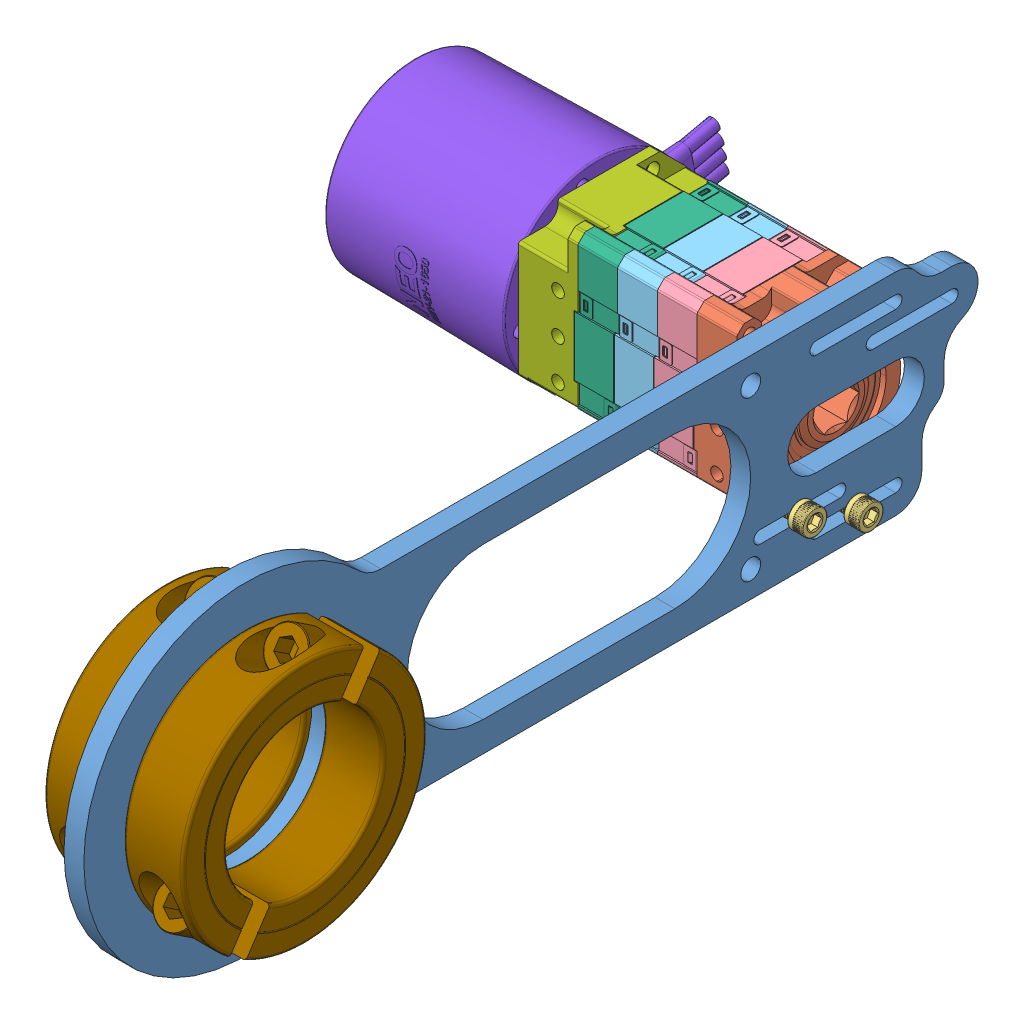
SolidWorks assembly motor to shaft mount, configuration Default. Lengths in mm.
Overall size (159.95 108.01 301.97).
11 component instances, 9 part files, 27 mates.
Components (placement in the parent):
- tubetomotormount-1: tubetomotormount [Default] at (115.7912 149.33 248.329) size (6.35 103.4 285.88)
- REV-21-2104.step-1: REV-21-2104.step [Default] at (103.0912 149.33 53.1781) x (1 0 0) z (0 1 0) size (23.2 50.8 61.92)
- 91251A342_Black-Oxide Alloy Steel Socket Head Screw (1)-1: 91251A342_Black-Oxide Alloy Steel Socket Head Screw (1) [91251A342] at (115.0292 123.93 53.1781) x (0 1 0) z (1 0 0) size (7.94 7.94 17.97)
- 91251A342_Black-Oxide Alloy Steel Socket Head Screw (1)-3: 91251A342_Black-Oxide Alloy Steel Socket Head Screw (1) [91251A342] at (115.0292 131.3695 71.1386) x (0 1 0) z (1 0 0) size (7.94 7.94 17.97)
- REV-21-2101.step1-1: REV-21-2101.step1 [Default] at (87.2162 149.3255 53.1781) x (0 1 0) z (1 0 0) size (61.91 50.8 16.85)
- REV-21-2102.step-1: REV-21-2102.step [Default] at (74.5162 149.3255 53.1781) x (0 1 0) z (1 0 0) size (61.91 50.8 16.85)
- REV-21-2103.step-1: REV-21-2103.step [Default] at (61.8162 149.3255 53.1781) x (0 1 0) z (1 0 0) size (61.91 50.8 16.85)
- REV-21-2106.step-1: REV-21-2106.step [Default] at (45.9412 149.3255 53.1781) x (0 1 0) z (1 0 0) size (61.91 50.8 19.05)
- REV-21-1650-V1.1.step-1: REV-21-1650-V1.1.step [Default] at (36.4162 149.3255 53.1781) x (0 -0.832107 0.554615) z (1 0 0) size (68.13 68.01 93.35)
- 6063K26_Clamping Two-Piece Shaft Collar-1: 6063K26_Clamping Two-Piece Shaft Collar [6063K26] at (103.1162 149.33 248.329) x (0 -0.83294 0.553363) z (-1 0 0) size (77.86 78 19.11)
- 6063K26_Clamping Two-Piece Shaft Collar-2: 6063K26_Clamping Two-Piece Shaft Collar [6063K26] at (128.4662 149.33 248.329) x (0 -0.83294 0.553363) z (-1 0 0) size (77.86 78 19.11)
Mates (geometry in assembly coordinates):
- Parallel1: parallel anti-aligned: plane of REV-21-2104.step-1 through (103.0912 149.33 53.1781) normal (0 0 -1)
- Concentric14: concentric anti-aligned: cylinder of REV-21-2104.step-1 through (112.6162 123.93 53.1781) axis (1 0 0) radius 2.0193; circle of 91251A342_Black-Oxide Alloy Steel Socket Head Screw (1)-1
- Coincident21: coincident anti-aligned: plane of tubetomotormount-1 through (118.9662 149.33 248.329) normal (1 0 0); plane of 91251A342_Black-Oxide Alloy Steel Socket Head Screw (1)-1 through (118.9662 120.2025 53.1781) normal (-1 0 0)
- Coincident22: coincident anti-aligned: plane of tubetomotormount-1 through (112.6162 149.33 248.329) normal (-1 0 0); plane of REV-21-2104.step-1 through (112.6162 149.33 53.1781) normal (1 0 0)
- Concentric17: concentric anti-aligned: cylinder of REV-21-2104.step-1 through (112.6162 131.3695 71.1386) axis (1 0 0) radius 2.0193; circle of 91251A342_Black-Oxide Alloy Steel Socket Head Screw (1)-3
- Coincident25: coincident anti-aligned: plane of tubetomotormount-1 through (118.9662 149.33 248.329) normal (1 0 0); plane of 91251A342_Black-Oxide Alloy Steel Socket Head Screw (1)-3 through (118.9662 127.642 71.1386) normal (-1 0 0)
- Concentric18: concentric anti-aligned: cylinder of REV-21-2104.step-1 through (93.5662 122.338 31.7468) axis (-1 0 0) radius 2.0193; cylinder of REV-21-2101.step-1 through (93.5662 122.338 31.7468) axis (1 0 0) radius 2.5
- Coincident26: coincident anti-aligned: plane of REV-21-2104.step-1 through (93.5662 149.33 53.1781) normal (-1 0 0); plane of REV-21-2101.step-1 through (93.5662 149.3255 53.1781) normal (1 0 0)
- Coincident27: coincident aligned: plane of REV-21-2104.step-1 through (93.5662 123.93 78.5781) normal (0 0 1); plane of REV-21-2101.step-1 through (93.5662 174.7255 78.5781) normal (0 0 1)
- Coincident29: coincident anti-aligned: plane of REV-21-2101.step-1 through (80.8662 149.3255 53.1781) normal (-1 0 0); plane of REV-21-2102.step-1 through (80.8662 149.3255 53.1781) normal (1 0 0)
- Concentric26: concentric aligned: cylinder of REV-21-2101.step-1 through (93.5662 176.313 74.6093) axis (1 0 0) radius 2.5; cylinder of REV-21-2102.step-1 through (80.8662 176.313 74.6093) axis (1 0 0) radius 2.5
- Concentric27: concentric aligned: cylinder of REV-21-2101.step-1 through (93.5662 122.338 31.7468) axis (1 0 0) radius 2.5; cylinder of REV-21-2102.step-1 through (80.8662 122.338 31.7468) axis (1 0 0) radius 2.5
- Coincident30: coincident anti-aligned: plane of REV-21-2102.step-1 through (68.1662 149.3255 53.1781) normal (-1 0 0); plane of REV-21-2103.step-1 through (68.1662 149.3255 53.1781) normal (1 0 0)
- Concentric28: concentric aligned: cylinder of REV-21-2102.step-1 through (80.8662 176.313 74.6093) axis (1 0 0) radius 2.5; cylinder of REV-21-2103.step-1 through (68.1662 176.313 74.6093) axis (1 0 0) radius 2.5
- Concentric29: concentric aligned: cylinder of REV-21-2102.step-1 through (80.8662 122.338 31.7468) axis (1 0 0) radius 2.5; cylinder of REV-21-2103.step-1 through (68.1662 122.338 31.7468) axis (1 0 0) radius 2.5
- Coincident31: coincident anti-aligned: plane of REV-21-2103.step-1 through (55.4662 149.3255 53.1781) normal (-1 0 0); plane of REV-21-2106.step-1 through (55.4662 149.3255 53.1781) normal (1 0 0)
- Concentric30: concentric anti-aligned: cylinder of REV-21-2103.step-1 through (68.1662 176.313 74.6093) axis (1 0 0) radius 2.5; cylinder of REV-21-2106.step-1 through (55.4662 176.313 74.6093) axis (-1 0 0) radius 2.5
- Concentric31: concentric anti-aligned: cylinder of REV-21-2103.step-1 through (68.1662 122.338 31.7468) axis (1 0 0) radius 2.5; cylinder of REV-21-2106.step-1 through (55.4662 122.338 31.7468) axis (-1 0 0) radius 2.5
- Concentric34: concentric anti-aligned: cylinder of REV-21-2106.step-1 through (55.4662 128.19 67.2653) axis (-1 0 0) radius 2.5; cylinder of REV-21-1650-V1.1.step-1 through (36.4162 128.19 67.2653) axis (1 0 0) radius 2.0193
- Concentric35: concentric anti-aligned: cylinder of REV-21-2106.step-1 through (55.4662 170.461 39.0909) axis (-1 0 0) radius 2.5; cylinder of REV-21-1650-V1.1.step-1 through (36.4162 170.461 39.0909) axis (1 0 0) radius 2.0193
- Coincident32: coincident anti-aligned: plane of REV-21-2106.step-1 through (36.4162 149.3255 53.1781) normal (-1 0 0); plane of REV-21-1650-V1.1.step-1 through (36.4162 149.3255 53.1781) normal (1 0 0)
- Concentric37: concentric anti-aligned: cylinder of tubetomotormount-1 through (118.9662 149.33 248.329) axis (-1 0 0) radius 27.5; cylinder of 6063K26_Clamping Two-Piece Shaft Collar-1 through (93.6162 149.33 248.329) axis (1 0 0) radius 25
- Coincident33: coincident anti-aligned: plane of tubetomotormount-1 through (112.6162 149.33 248.329) normal (-1 0 0); plane of 6063K26_Clamping Two-Piece Shaft Collar-1 through (112.6162 149.33 248.329) normal (1 0 0)
- Tangent3: tangent anti-aligned: plane of tubetomotormount-1 through (118.9662 165.2712 248.329) normal (0 1 0); cylinder of REV-21-2104.step-1 through (112.6162 167.2905 35.2176) axis (1 0 0) radius 2.0193
- Coincident36: coincident anti-aligned: plane of tubetomotormount-1 through (118.9662 149.33 248.329) normal (1 0 0); plane of 6063K26_Clamping Two-Piece Shaft Collar-2 through (118.9662 149.33 248.329) normal (-1 0 0)
- Concentric39: concentric anti-aligned: cylinder of tubetomotormount-1 through (118.9662 149.33 248.329) axis (-1 0 0) radius 27.5; cylinder of 6063K26_Clamping Two-Piece Shaft Collar-2 through (118.9662 149.33 248.329) axis (1 0 0) radius 25
- Coincident37: coincident aligned: plane of 6063K26_Clamping Two-Piece Shaft Collar-1 through (93.6162 126.9428 259.4562) normal (0 0.553363 0.83294); plane of 6063K26_Clamping Two-Piece Shaft Collar-2 through (118.9662 126.9428 259.4562) normal (0 0.553363 0.83294)
